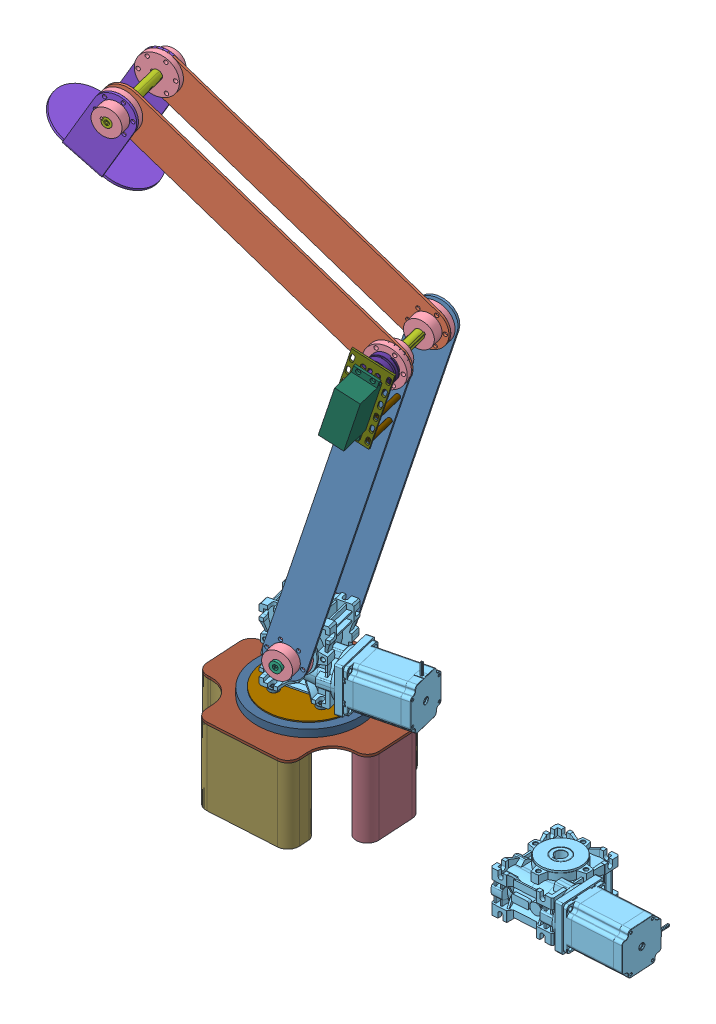
SolidWorks assembly Arm Assembly3, configuration Default. Lengths in mm.
Overall size (729.54 813.81 228.91).
36 component instances, 18 part files, 93 mates.
Components (placement in the parent):
- Link 2-1: Link 2 [Default] at (46.1819 312.4393 295.2651) x (0.276658 0.958565 -0.06792) z (0.238421 0 0.971162) size (457.2 50.8 3.17)
- Link 3-1: Link 3 [Default] at (168.993 730.6018 354.4422) x (-0.816914 0.540768 0.200553) z (0.238421 0 0.971162) size (406.4 50.8 3.17)
- Flanged Bearing-1: Flanged Bearing [Default] at (-150.7554 901.5329 364.2098) x (0.971162 0 -0.238421) z (0.238421 0 0.971162) size (38.1 38.1 12.7)
- Keyed hub-1: Keyed hub [Default] at (41.8754 319.6751 379.8434) x (0.225868 -0.972578 -0.055451) z (-0.944531 -0.232575 0.231883) size (50.8 25.4 50.8)
- Link 2-2: Link 2 [Default] at (67.4132 312.4393 381.7471) x (0.276658 0.958565 -0.06792) z (0.238421 0 0.971162) size (457.2 50.8 3.17)
- Link 3-2: Link 3 [Default] at (152.3036 730.6018 286.4609) x (-0.816914 0.540768 0.200553) z (0.238421 0 0.971162) size (406.4 50.8 3.17)
- Flanged Bearing-3: Flanged Bearing [Default] at (-134.8593 901.5329 428.9596) x (-0.897412 -0.382247 0.220315) z (-0.238421 0 -0.971162) size (38.1 38.1 12.7)
- Keyed hub-2: Keyed hub [Default] at (137.0717 709.236 282.0271) x (0.444882 -0.888904 -0.109219) z (-0.86327 -0.458093 0.211933) size (50.8 25.4 50.8)
- Keyed hub-3: Keyed hub [Default] at (25.1859 319.6751 311.8621) x (-0.225868 0.972578 0.055451) z (-0.944531 -0.232575 0.231883) size (50.8 25.4 50.8)
- Keyed hub-4: Keyed hub [Default] at (158.3031 709.236 368.5091) x (-0.444882 0.888904 0.109219) z (-0.86327 -0.458093 0.211933) size (50.8 25.4 50.8)
- Flanged Bearing-4: Flanged Bearing [Default] at (134.9522 709.236 273.3935) x (0.894281 0.38995 -0.219546) z (-0.238421 0 -0.971162) size (38.1 38.1 12.7)
- Nema Stepper Motor-2: Nema Stepper Motor [Default] at (106.1749 300.7059 328.0186) x (0.971162 0 -0.238421) z (-0.238421 0 -0.971162) size (171.01 100.01 63.01)
- Nema Stepper Motor-3: Nema Stepper Motor [Default] at (426.1519 175.0272 335.1941) x (0.998228 0 -0.059501) z (0 -1 0) size (171.01 100.01 63.01)
- Keyed Drive Shaft-1: Keyed Drive Shaft [Default] at (6.1624 318.2407 219.9212) x (0.225868 -0.972578 -0.055451) z (0.238421 0 0.971162) size (19.9 19.9 128.01)
- Keyed Shaft-1: Keyed Shaft [Default] at (131.7338 709.236 260.284) x (0.444882 -0.888904 -0.109219) z (0.238421 0 0.971162) size (12.7 12.5 104.14)
- Link 4-1: Link 4 [Default] at (-199.0226 846.4761 418.7799) x (0.238421 0 0.971162) z (-0.849206 0.485165 0.20848) size (90.37 102.6 133.86)
- Keyed hub-5: Keyed hub [Default] at (-148.9877 901.5329 371.4103) x (-0.471173 -0.874423 0.115673) z (0.849206 -0.485165 -0.20848) size (50.8 25.4 50.8)
- Keyed hub-6: Keyed hub [Default] at (-132.7397 901.5329 437.5933) x (0.471173 0.874423 -0.115673) z (0.849206 -0.485165 -0.20848) size (50.8 25.4 50.8)
- Keyed Shaft-2: Keyed Shaft [Default] at (-124.2615 901.5329 472.1278) x (-0.471173 -0.874423 0.115673) z (-0.238421 0 -0.971162) size (12.7 12.5 104.14)
- Bearing maybe-1: Bearing maybe [Default] at (32.1724 257.1751 346.1862) x (0.971162 0 -0.238421) z (0.238421 0 0.971162) size (117.56 1.5 117.56)
- Bearing other part-1: Bearing other part [Default] at (32.1724 247.1751 346.1862) size (140 10 140)
- Top base plate-1: Top base plate [Default] at (33.5723 244.0001 346.2554) x (0.998228 0 -0.059501) z (0.059501 0 0.998228) size (222 3.17 194.94)
- arm base spacer large part-1: arm base spacer large part [Default] at (32.1724 142.4001 346.1862) x (-0.998228 0 0.059501) z (-0.059501 0 -0.998228) size (171.5 101.6 195.24)
- arm base spacer small part-1: arm base spacer small part [Default] at (130.8381 142.4001 364.6329) x (0.998228 0 -0.059501) z (0.059501 0 0.998228) size (30 101.6 78.26)
- 4 mm M6 spacer-1: 4 mm M6 spacer [94669A162] at (64.993 260.6751 360.782) x (-1 0 0) z (0 -1 0) size (13 13 4)
- 4 mm M6 spacer-2: 4 mm M6 spacer [94669A162] at (12.5502 260.6751 373.6567) x (1 0 0) z (0 -1 0) size (13 13 4)
- 4 mm M6 spacer-3: 4 mm M6 spacer [94669A162] at (54.5025 260.6751 318.0509) x (1 0 0) z (0 -1 0) size (13 13 4)
- 4 mm M6 spacer-4: 4 mm M6 spacer [94669A162] at (2.0597 260.6751 330.9256) x (1 0 0) z (0 -1 0) size (13 13 4)
- 80 kg-1: 80 kg [Default] at (147.8814 663.6637 448.4969) x (0.276658 0.958565 -0.06792) z (-0.930922 0.284873 0.228542) size (82 48 30)
- servo plate-1: servo plate [Default] at (160.2556 689.9235 403.7565) x (0.276658 0.958565 -0.06792) z (-0.930922 0.284873 0.228542) size (101.6 2.54 50.8)
- 2764K312_Servomotor Precision Flexible Shaft Coupling-1: 2764K312_Servomotor Precision Flexible Shaft Coupling [2764K312] at (161.4643 709.236 381.3855) x (0.971162 0 -0.238421) z (0.238421 0 0.971162) size (34.04 34.04 37.8)
- Flanged Bearing-5: Flanged Bearing [Default] at (156.1835 709.236 359.8755) x (0.813188 0.54669 -0.199638) z (-0.238421 0 -0.971162) size (38.1 38.1 12.7)
- 91125A471_Female Threaded Round Standoff-1: 91125A471_Female Threaded Round Standoff [91125A471] at (123.489 655.9301 390.5516) x (0.971162 0 -0.238421) z (0.238421 0 0.971162) size (6.35 6.35 38.54)
- 91125A471_Female Threaded Round Standoff-2: 91125A471_Female Threaded Round Standoff [91125A471] at (172.6473 675.3409 378.797) x (-0.144728 0.988833 0.035531) z (-0.238421 0 -0.971162) size (6.35 6.35 38.54)
- 91125A471_Female Threaded Round Standoff-4: 91125A471_Female Threaded Round Standoff [91125A471] at (132.7587 687.5952 388.5897) x (-0.310292 0.947584 0.076177) z (-0.238421 0 -0.971162) size (6.35 6.35 38.54)
- 91125A471_Female Threaded Round Standoff-6: 91125A471_Female Threaded Round Standoff [91125A471] at (163.5722 643.7523 381.025) x (-0.466934 0.87683 0.114633) z (-0.238421 0 -0.971162) size (6.35 6.35 38.54)
Mates (geometry in assembly coordinates):
- Concentric3: concentric aligned: cylinder of Keyed hub-1 through (43.7678 319.6751 387.552) axis (0.238421 0 0.971162) radius 17.4625; cylinder of Link 2-2 through (43.7678 319.6751 387.552) axis (0.238421 0 0.971162) radius 17.4625
- Coincident2: coincident anti-aligned: plane of Keyed hub-1 through (43.7678 319.6751 387.552) normal (0.238421 0 0.971162); plane of Link 2-2 through (43.7678 319.6751 387.552) normal (-0.238421 0 -0.971162)
- Concentric4: concentric aligned: cylinder of Keyed hub-1 through (48.5296 299.1712 386.383) axis (0.238421 0 0.971162) radius 2.5527; cylinder of Link 2-2 through (49.2866 299.1712 389.4665) axis (0.238421 0 0.971162) radius 2.5527
- Concentric5: concentric anti-aligned: cylinder of Link 2-1 through (22.5365 319.6751 301.0701) axis (0.238421 0 0.971162) radius 17.4625; cylinder of Keyed hub-3 through (23.2934 319.6751 304.1535) axis (-0.238421 0 -0.971162) radius 17.4625
- Coincident3: coincident anti-aligned: plane of Link 2-1 through (23.2934 319.6751 304.1535) normal (0.238421 0 0.971162); plane of Keyed hub-3 through (23.2934 319.6751 304.1535) normal (-0.238421 0 -0.971162)
- Concentric7: concentric anti-aligned: cylinder of Link 2-1 through (3.6677 325.6808 308.9716) axis (0.238421 0 0.971162) radius 2.5527; cylinder of Keyed hub-3 through (3.6677 325.6808 308.9716) axis (-0.238421 0 -0.971162) radius 2.5527
- Concentric8: concentric anti-aligned: cylinder of Keyed hub-1 through (41.8754 319.6751 379.8434) axis (0.238421 0 0.971162) radius 6.35; cylinder of Keyed hub-3 through (25.1859 319.6751 311.8621) axis (-0.238421 0 -0.971162) radius 6.35
- Coincident5: coincident aligned: plane of Keyed hub-1 through (41.5168 321.2191 379.9315) normal (0.225868 -0.972578 -0.055451); plane of Keyed hub-3 through (24.8273 321.2191 311.9501) normal (0.225868 -0.972578 -0.055451)
- Concentric10: concentric anti-aligned: cylinder of Link 2-1 through (134.9703 709.236 273.4675) axis (0.238421 0 0.971162) radius 17.4625; cylinder of Flanged Bearing-4 through (133.4382 709.236 267.2266) axis (-0.238421 0 -0.971162) radius 17.4625
- Concentric11: concentric anti-aligned: cylinder of Link 3-1 through (155.6536 709.236 357.7171) axis (0.238421 0 0.971162) radius 17.4625; cylinder of Keyed hub-4 through (156.4106 709.236 360.8005) axis (-0.238421 0 -0.971162) radius 17.4625
- Coincident8: coincident anti-aligned: plane of Link 3-1 through (156.4106 709.236 360.8005) normal (0.238421 0 0.971162); plane of Keyed hub-4 through (156.4106 709.236 360.8005) normal (-0.238421 0 -0.971162)
- Concentric12: concentric anti-aligned: cylinder of Link 3-1 through (167.4823 726.9696 358.0824) axis (0.238421 0 0.971162) radius 2.5527; cylinder of Keyed hub-4 through (167.4823 726.9696 358.0824) axis (-0.238421 0 -0.971162) radius 2.5527
- Concentric13: concentric aligned: cylinder of Link 3-2 through (138.9642 709.236 289.7357) axis (0.238421 0 0.971162) radius 17.4625; cylinder of Keyed hub-2 through (138.9642 709.236 289.7357) axis (0.238421 0 0.971162) radius 17.4625
- Coincident9: coincident anti-aligned: plane of Link 3-2 through (138.9642 709.236 289.7357) normal (-0.238421 0 -0.971162); plane of Keyed hub-2 through (138.9642 709.236 289.7357) normal (0.238421 0 0.971162)
- Concentric14: concentric aligned: cylinder of Link 3-2 through (150.7929 726.9696 290.1011) axis (0.238421 0 0.971162) radius 2.5527; cylinder of Keyed hub-2 through (150.0359 726.9696 287.0176) axis (0.238421 0 0.971162) radius 2.5527
- Concentric15: concentric anti-aligned: cylinder of Keyed hub-2 through (137.0717 709.236 282.0271) axis (0.238421 0 0.971162) radius 6.35; cylinder of Keyed hub-4 through (158.3031 709.236 368.5091) axis (-0.238421 0 -0.971162) radius 6.35
- Coincident10: coincident aligned: plane of Keyed hub-2 through (137.778 707.8249 281.8537) normal (-0.444882 0.888904 0.109219); plane of Keyed hub-4 through (159.0093 707.8249 368.3357) normal (-0.444882 0.888904 0.109219)
- Concentric17: concentric aligned: cylinder of Flanged Bearing-1 through (-149.2414 901.5329 370.3766) axis (0.238421 0 0.971162) radius 17.4625; cylinder of Link 3-2 through (-151.5306 901.5329 361.0523) axis (0.238421 0 0.971162) radius 17.4625
- Coincident13: coincident anti-aligned: plane of Flanged Bearing-1 through (-151.5306 918.9954 361.0523) normal (0.238421 0 0.971162); plane of Link 3-2 through (138.9642 709.236 289.7357) normal (-0.238421 0 -0.971162)
- Concentric18: concentric anti-aligned: cylinder of Link 3-1 through (-134.8411 901.5329 429.0336) axis (0.238421 0 0.971162) radius 17.4625; cylinder of Flanged Bearing-3 through (-136.3732 901.5329 422.7928) axis (-0.238421 0 -0.971162) radius 17.4625
- Coincident14: coincident anti-aligned: plane of Link 3-1 through (156.4106 709.236 360.8005) normal (0.238421 0 0.971162); plane of Flanged Bearing-3 through (-140.5666 917.6693 433.7085) normal (-0.238421 0 -0.971162)
- Concentric21: concentric anti-aligned: cylinder of Keyed hub-1 through (41.8754 319.6751 379.8434) axis (0.238421 0 0.971162) radius 6.35; cylinder of Keyed Drive Shaft-1 through (48.7896 319.6751 408.0071) axis (-0.238421 0 -0.971162) radius 7
- Parallel1: parallel anti-aligned: plane of Keyed hub-1 through (41.5168 321.2191 379.9315) normal (0.225868 -0.972578 -0.055451); plane of Keyed Drive Shaft-1 through (37.972 323.3392 344.7624) normal (-0.225868 0.972578 0.055451)
- Coincident18: coincident anti-aligned: plane of Keyed hub-3 through (25.1859 319.6751 311.8621) normal (0.238421 0 0.971162); plane of Keyed Drive Shaft-1 through (31.2369 322.3989 310.3766) normal (-0.238421 0 -0.971162)
- Coincident19: coincident anti-aligned: plane of Keyed hub-1 through (41.8754 319.6751 379.8434) normal (-0.238421 0 -0.971162); plane of Keyed Drive Shaft-1 through (47.9263 322.3989 378.3579) normal (0.238421 0 0.971162)
- Concentric22: concentric anti-aligned: cylinder of Keyed hub-2 through (137.0717 709.236 282.0271) axis (0.238421 0 0.971162) radius 6.35; cylinder of Keyed Shaft-1 through (158.9853 709.236 371.2878) axis (-0.238421 0 -0.971162) radius 6.35
- Coincident20: coincident aligned: plane of Keyed hub-2 through (137.778 707.8249 281.8537) normal (-0.444882 0.888904 0.109219); plane of Keyed Shaft-1 through (163.7919 710.0007 370.1078) normal (-0.444882 0.888904 0.109219)
- Coincident22: coincident anti-aligned: plane of Link 2-1 through (23.2934 319.6751 304.1535) normal (0.238421 0 0.971162); plane of Flanged Bearing-4 through (142.3405 693.1559 274.9274) normal (-0.238421 0 -0.971162)
- Distance1: distance = 2.54 mm anti-aligned: plane of Flanged Bearing-4 through (140.8236 698.6407 278.4906) normal (0.238421 0 0.971162); plane of Keyed hub-2 through (137.0717 709.236 282.0271) normal (-0.238421 0 -0.971162)
- Concentric23: concentric anti-aligned: cylinder of Link 4-1 through (-130.0903 901.5329 448.3853) axis (-0.238421 0 -0.971162) radius 17.4625; cylinder of Keyed hub-6 through (-130.8472 901.5329 445.3019) axis (0.238421 0 0.971162) radius 17.4625
- Concentric24: concentric anti-aligned: cylinder of Link 4-1 through (-141.385 919.6081 447.8889) axis (-0.238421 0 -0.971162) radius 2.5527; cylinder of Keyed hub-6 through (-141.385 919.6081 447.8889) axis (0.238421 0 0.971162) radius 2.5527
- Coincident27: coincident anti-aligned: plane of Link 4-1 through (-208.3309 810.6124 464.3242) normal (-0.238421 0 -0.971162); plane of Keyed hub-6 through (-130.8472 901.5329 445.3019) normal (0.238421 0 0.971162)
- Concentric25: concentric anti-aligned: cylinder of Link 4-1 through (-151.6371 901.5329 360.6183) axis (0.238421 0 0.971162) radius 17.4625; cylinder of Keyed hub-5 through (-150.8801 901.5329 363.7017) axis (-0.238421 0 -0.971162) radius 17.4625
- Concentric26: concentric anti-aligned: cylinder of Link 4-1 through (-161.4179 919.6081 366.2888) axis (0.238421 0 0.971162) radius 2.5527; cylinder of Keyed hub-5 through (-161.4179 919.6081 366.2888) axis (-0.238421 0 -0.971162) radius 2.5527
- Concentric27: concentric anti-aligned: cylinder of Keyed hub-5 through (-148.9877 901.5329 371.4103) axis (-0.238421 0 -0.971162) radius 6.35; cylinder of Keyed Shaft-2 through (-151.513 901.5329 361.124) axis (0.238421 0 0.971162) radius 6.35
- Coincident31: coincident aligned: plane of Keyed hub-5 through (-148.2397 902.9211 371.2267) normal (-0.471173 -0.874423 0.115673); plane of Keyed Shaft-2 through (-154.7985 905.2255 361.9306) normal (-0.471173 -0.874423 0.115673)
- Coincident32: coincident aligned: plane of Keyed hub-6 through (-126.6838 901.5329 462.2608) normal (0.238421 0 0.971162); plane of Keyed Shaft-2 through (-126.6838 901.5329 462.2608) normal (0.238421 0 0.971162)
- Coincident34: coincident anti-aligned: plane of Link 4-1 through (-228.3638 810.6124 382.724) normal (0.238421 0 0.971162); plane of Keyed hub-5 through (-150.8801 901.5329 363.7017) normal (-0.238421 0 -0.971162)
- Coincident36: coincident aligned: plane of Keyed hub-6 through (-133.4877 900.1448 437.7769) normal (0.471173 0.874423 -0.115673); plane of Keyed Shaft-2 through (-156.2945 902.4492 362.2979) normal (0.471173 0.874423 -0.115673)
- Concentric28: concentric anti-aligned: cone of Flanged Bearing-3 through (-133.505 901.5329 434.4762) axis (-0.238421 0 -0.971162); cylinder of Keyed Shaft-2 through (-151.513 901.5329 361.124) axis (0.238421 0 0.971162) radius 6.35
- Distance3: distance = 2.54 mm anti-aligned: plane of Flanged Bearing-3 through (-137.6167 912.1654 436.1751) normal (0.238421 0 0.971162); plane of Keyed hub-6 through (-132.7397 901.5329 437.5933) normal (-0.238421 0 -0.971162)
- Coincident37: coincident anti-aligned: plane of Bearing maybe-1 through (32.1724 257.1751 346.1862) normal (0 -1 0); plane of Bearing other part-1 through (32.1724 257.1751 346.1862) normal (0 1 0)
- Concentric29: concentric aligned: cylinder of Bearing maybe-1 through (32.1724 258.6751 346.1862) axis (0 -1 0) radius 58.7822; cylinder of Bearing other part-1 through (32.1724 257.1751 346.1862) axis (0 -1 0) radius 70
- Coincident38: coincident anti-aligned: plane of Top base plate-1 through (74.0847 244.0001 261.2257) normal (0 -1 0); plane of arm base spacer small part-1 through (130.8381 244.0001 364.6329) normal (0 1 0)
- Coincident40: coincident anti-aligned: plane of Top base plate-1 through (74.0847 244.0001 261.2257) normal (0 -1 0); plane of arm base spacer large part-1 through (32.1724 244.0001 346.1862) normal (0 1 0)
- Coincident45: coincident anti-aligned: plane of Bearing other part-1 through (32.1724 247.1751 346.1862) normal (0 -1 0); plane of Top base plate-1 through (74.0847 247.1751 261.2257) normal (0 1 0)
- Concentric32: concentric aligned: cylinder of Bearing other part-1 through (32.1724 257.1751 346.1862) axis (0 -1 0) radius 70; circle of arm base spacer large part-1
- Coincident50: coincident anti-aligned: plane of Bearing maybe-1 through (32.1724 258.6751 346.1862) normal (0 1 0); plane of 4 mm M6 spacer-3 through (54.5025 258.6751 318.0509) normal (0 -1 0)
- Coincident55: coincident anti-aligned: plane of Nema Stepper Motor-2 through (106.1749 300.7059 328.0186) normal (-0.238421 0 -0.971162); plane of Bearing maybe-1 through (32.1724 257.1751 346.1862) normal (0.238421 0 0.971162)
- Distance5: distance = 76.2 mm aligned: plane of Nema Stepper Motor-2 through (106.1749 300.7059 328.0186) normal (0.971162 0 -0.238421); plane of Bearing maybe-1 through (32.1724 257.1751 346.1862) normal (0.971162 0 -0.238421)
- Coincident57: coincident aligned: plane of Top base plate-1 through (-6.0476 247.1751 446.2586) normal (0.059501 0 0.998228); plane of arm base spacer large part-1 through (84.7912 244.0001 440.844) normal (0.059501 0 0.998228)
- Coincident58: coincident aligned: plane of Top base plate-1 through (-75.7951 247.1751 376.9496) normal (-0.998228 0 0.059501); plane of arm base spacer large part-1 through (-75.8042 244.0001 376.7975) normal (-0.998228 0 0.059501)
- Concentric37: concentric aligned: cylinder of Top base plate-1 through (130.8381 247.1751 364.6329) axis (0 -1 0) radius 15; cylinder of arm base spacer small part-1 through (130.8381 244.0001 364.6329) axis (0 -1 0) radius 15
- Coincident59: coincident aligned: plane of Top base plate-1 through (145.8116 247.1751 363.7404) normal (0.998228 0 -0.059501); plane of arm base spacer small part-1 through (145.8116 244.0001 363.7404) normal (0.998228 0 -0.059501)
- Parallel2: parallel aligned: plane of Nema Stepper Motor-3 through (350.3499 203.0272 320.7095) normal (0 1 0); plane of Top base plate-1 through (74.0847 247.1751 261.2257) normal (0 1 0)
- Parallel3: parallel anti-aligned: plane of Nema Stepper Motor-3 through (312.2058 175.0272 353.0364) normal (-0.998228 0 0.059501); plane of arm base spacer small part-1 through (145.8116 244.0001 363.7404) normal (0.998228 0 -0.059501)
- Coincident61: coincident anti-aligned: plane of Nema Stepper Motor-2 through (79.0486 262.6751 363.5095) normal (0 -1 0); plane of 4 mm M6 spacer-1 through (64.993 262.6751 360.782) normal (0 1 0)
- Concentric39: concentric aligned: cylinder of Nema Stepper Motor-2 through (64.993 359.6751 360.782) axis (0 -1 0) radius 3.25; cylinder of 4 mm M6 spacer-1 through (64.993 262.6751 360.782) axis (0 -1 0) radius 3.15
- Coincident62: coincident anti-aligned: plane of Bearing maybe-1 through (32.1724 258.6751 346.1862) normal (0 1 0); plane of 4 mm M6 spacer-1 through (64.993 258.6751 360.782) normal (0 -1 0)
- Concentric40: concentric aligned: cylinder of Nema Stepper Motor-2 through (54.5025 359.6751 318.0509) axis (0 -1 0) radius 3.25; cylinder of 4 mm M6 spacer-3 through (54.5025 262.6751 318.0509) axis (0 -1 0) radius 3.15
- Concentric41: concentric aligned: cylinder of Nema Stepper Motor-2 through (2.0597 359.6751 330.9256) axis (0 -1 0) radius 3.25; cylinder of 4 mm M6 spacer-4 through (2.0597 262.6751 330.9256) axis (0 -1 0) radius 3.15
- Concentric42: concentric aligned: cylinder of Nema Stepper Motor-2 through (12.5502 359.6751 373.6567) axis (0 -1 0) radius 3.25; cylinder of 4 mm M6 spacer-2 through (12.5502 262.6751 373.6567) axis (0 -1 0) radius 3.15
- Concentric43: concentric aligned: cylinder of Keyed hub-1 through (43.7678 319.6751 387.552) axis (0.238421 0 0.971162) radius 17.4625; cylinder of Nema Stepper Motor-2 through (11.423 319.6751 255.8014) axis (0.238421 0 0.971162) radius 7
- Coincident65: coincident anti-aligned: plane of Nema Stepper Motor-2 through (41.0366 319.6751 376.4454) normal (0.238421 0 0.971162); plane of Keyed Drive Shaft-1 through (41.0409 319.6751 376.4444) normal (-0.238421 0 -0.971162)
- Coincident69: coincident anti-aligned: plane of 80 kg-1 through (138.2254 663.6637 409.1649) normal (-0.238421 0 -0.971162); plane of servo plate-1 through (160.2556 689.9235 403.7565) normal (0.238421 0 0.971162)
- Concentric48: concentric aligned: cylinder of 80 kg-1 through (173.2985 728.9116 442.257) axis (-0.238421 0 -0.971162) radius 3; cylinder of servo plate-1 through (163.6424 728.9116 402.925) axis (-0.238421 0 -0.971162) radius 3.302
- Concentric49: concentric aligned: cylinder of 80 kg-1 through (189.1242 724.0688 438.3718) axis (-0.238421 0 -0.971162) radius 3; cylinder of servo plate-1 through (179.4681 724.0688 399.0398) axis (-0.238421 0 -0.971162) radius 3.302
- Concentric50: concentric aligned: cylinder of 80 kg-1 through (152.5491 657.0192 447.351) axis (-0.238421 0 -0.971162) radius 3; cylinder of servo plate-1 through (142.8931 657.0192 408.019) axis (-0.238421 0 -0.971162) radius 3.302
- Concentric51: concentric aligned: cylinder of 80 kg-1 through (168.3748 652.1764 443.4658) axis (-0.238421 0 -0.971162) radius 3; cylinder of servo plate-1 through (158.7188 652.1764 404.1337) axis (-0.238421 0 -0.971162) radius 3.302
- Coincident71: coincident anti-aligned: plane of Link 2-2 through (44.5248 319.6751 390.6355) normal (0.238421 0 0.971162); plane of 2764K312_Servomotor Precision Flexible Shaft Coupling-1 through (156.9587 709.236 363.0329) normal (-0.238421 0 -0.971162)
- Concentric53: concentric anti-aligned: cylinder of Keyed Shaft-1 through (158.9853 709.236 371.2878) axis (-0.238421 0 -0.971162) radius 6.35; cylinder of 2764K312_Servomotor Precision Flexible Shaft Coupling-1 through (156.9587 709.236 363.0329) axis (0.238421 0 0.971162) radius 6.35
- Concentric54: concentric anti-aligned: cylinder of 80 kg-1 through (164.7873 709.236 394.9212) axis (0.238421 0 0.971162) radius 2; cylinder of 2764K312_Servomotor Precision Flexible Shaft Coupling-1 through (165.9698 709.236 399.7382) axis (-0.238421 0 -0.971162) radius 3.175
- Concentric55: concentric aligned: cone of Flanged Bearing-4 through (136.3065 709.236 278.9101) axis (-0.238421 0 -0.971162); cylinder of Keyed Shaft-1 through (158.9853 709.236 371.2878) axis (-0.238421 0 -0.971162) radius 6.35
- Concentric57: concentric anti-aligned: cylinder of Keyed Shaft-1 through (158.9853 709.236 371.2878) axis (-0.238421 0 -0.971162) radius 6.35; cylinder of 2764K312_Servomotor Precision Flexible Shaft Coupling-1 through (156.9587 709.236 363.0329) axis (0.238421 0 0.971162) radius 6.35
- Coincident73: coincident anti-aligned: plane of Keyed Shaft-1 through (158.9853 709.236 371.2878) normal (0.238421 0 0.971162); plane of 2764K312_Servomotor Precision Flexible Shaft Coupling-1 through (161.6273 680.822 370.6392) normal (-0.238421 0 -0.971162)
- Concentric58: concentric anti-aligned: cylinder of Link 2-2 through (156.2017 709.236 359.9495) axis (0.238421 0 0.971162) radius 17.4625; cylinder of Flanged Bearing-5 through (154.6696 709.236 353.7086) axis (-0.238421 0 -0.971162) radius 17.4625
- Coincident74: coincident anti-aligned: plane of Link 2-2 through (44.5248 319.6751 390.6355) normal (0.238421 0 0.971162); plane of Flanged Bearing-5 through (166.23 694.6141 360.7568) normal (-0.238421 0 -0.971162)
- Distance6: distance = 2.54 mm aligned: plane of Flanged Bearing-5 through (163.8064 699.6015 364.5426) normal (0.238421 0 0.971162); plane of Keyed hub-4 through (158.3031 709.236 368.5091) normal (0.238421 0 0.971162)
- Concentric59: concentric aligned: cylinder of Keyed Shaft-1 through (158.9853 709.236 371.2878) axis (-0.238421 0 -0.971162) radius 6.35; cone of Flanged Bearing-5 through (157.5378 709.236 365.392) axis (-0.238421 0 -0.971162)
- Coincident75: coincident anti-aligned: plane of servo plate-1 through (159.65 689.9235 401.2897) normal (-0.238421 0 -0.971162); plane of 2764K312_Servomotor Precision Flexible Shaft Coupling-1 through (165.9698 709.236 399.7382) normal (0.238421 0 0.971162)
- Parallel7: parallel anti-aligned: line of Link 2-2 through (68.1702 312.4393 384.8305) axis (0.276658 0.958565 -0.06792); line of servo plate-1 through (197.3496 731.3829 392.0344) axis (-0.276658 -0.958565 0.06792)
- Coincident76: coincident anti-aligned: plane of servo plate-1 through (159.65 689.9235 401.2897) normal (-0.238421 0 -0.971162); plane of 91125A471_Female Threaded Round Standoff-1 through (128.0309 655.9301 409.0522) normal (0.238421 0 0.971162)
- Coincident77: coincident anti-aligned: plane of Link 2-2 through (44.5248 319.6751 390.6355) normal (0.238421 0 0.971162); plane of 91125A471_Female Threaded Round Standoff-2 through (168.1054 675.3409 360.2964) normal (-0.238421 0 -0.971162)
- Coincident78: coincident anti-aligned: plane of Link 2-2 through (44.5248 319.6751 390.6355) normal (0.238421 0 0.971162); plane of 91125A471_Female Threaded Round Standoff-4 through (128.2168 687.5952 370.0891) normal (-0.238421 0 -0.971162)
- Coincident79: coincident anti-aligned: plane of Link 2-2 through (44.5248 319.6751 390.6355) normal (0.238421 0 0.971162); plane of 91125A471_Female Threaded Round Standoff-6 through (159.0303 643.7523 362.5243) normal (-0.238421 0 -0.971162)
- Parallel8: parallel anti-aligned: cylinder of 91125A471_Female Threaded Round Standoff-1 through (128.0309 655.9301 409.0522) axis (-0.238421 0 -0.971162) radius 3.175; cylinder of 91125A471_Female Threaded Round Standoff-6 through (159.0303 643.7523 362.5243) axis (0.238421 0 0.971162) radius 3.175
- Parallel9: parallel aligned: cylinder of 91125A471_Female Threaded Round Standoff-2 through (168.1054 675.3409 360.2964) axis (0.238421 0 0.971162) radius 3.175; cylinder of 91125A471_Female Threaded Round Standoff-4 through (128.2168 687.5952 370.0891) axis (0.238421 0 0.971162) radius 3.175
- Parallel10: parallel anti-aligned: cylinder of 91125A471_Female Threaded Round Standoff-1 through (128.0309 655.9301 409.0522) axis (-0.238421 0 -0.971162) radius 3.175; cylinder of 91125A471_Female Threaded Round Standoff-4 through (128.2168 687.5952 370.0891) axis (0.238421 0 0.971162) radius 3.175
- Parallel11: parallel aligned: cylinder of 91125A471_Female Threaded Round Standoff-2 through (168.1054 675.3409 360.2964) axis (0.238421 0 0.971162) radius 3.175; cylinder of 91125A471_Female Threaded Round Standoff-6 through (159.0303 643.7523 362.5243) axis (0.238421 0 0.971162) radius 3.175
- Concentric61: concentric anti-aligned: cylinder of Link 2-2 through (159.0606 643.7523 362.6477) axis (-0.238421 0 -0.971162) radius 1.972; cylinder of 91125A471_Female Threaded Round Standoff-6 through (159.0303 643.7523 362.5243) axis (0.238421 0 0.971162) radius 3.175
- Concentric62: concentric anti-aligned: cylinder of Link 2-2 through (168.1357 675.3409 360.4197) axis (-0.238421 0 -0.971162) radius 1.972; cylinder of 91125A471_Female Threaded Round Standoff-2 through (168.1054 675.3409 360.2964) axis (0.238421 0 0.971162) radius 3.175
- Concentric63: concentric anti-aligned: cylinder of Link 2-2 through (128.2471 687.5952 370.2124) axis (-0.238421 0 -0.971162) radius 1.972; cylinder of 91125A471_Female Threaded Round Standoff-4 through (128.2168 687.5952 370.0891) axis (0.238421 0 0.971162) radius 3.175
- Concentric64: concentric aligned: cylinder of Link 2-2 through (119.05 655.9301 372.4703) axis (-0.238421 0 -0.971162) radius 1.972; cylinder of 91125A471_Female Threaded Round Standoff-1 through (128.0309 655.9301 409.0522) axis (-0.238421 0 -0.971162) radius 3.175
